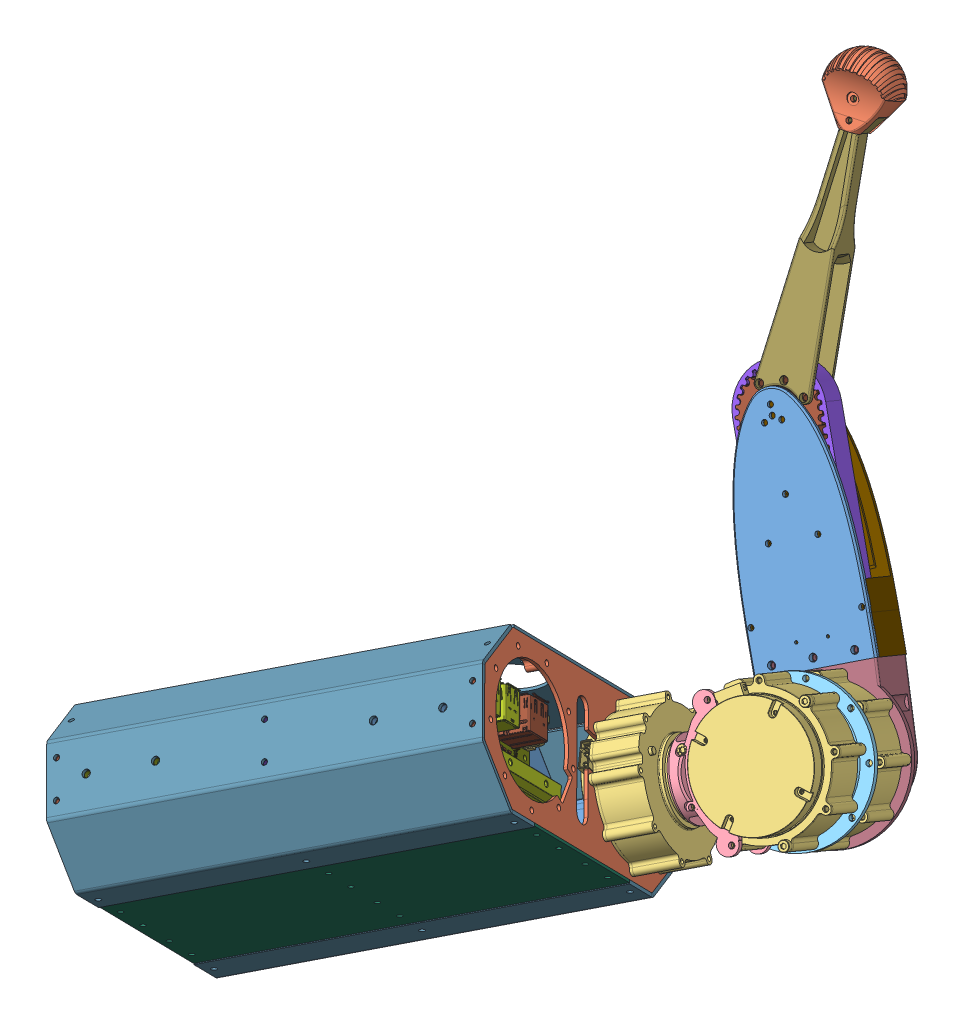
SolidWorks assembly OpenPaws, configuration 默认. Lengths in mm.
Overall size (320.72 417.64 440.55).
429 component instances, 92 part files, 82 mates.
Components (placement in the parent):
- BackFrame-1: BackFrame [默认] at (73.8698 29.661 407.5892) x (-0.005778 -0.713341 -0.700793) z (0.575051 -0.575706 0.581273) size (175.11 55 85)
- Shoulder-1: Shoulder [默认] at (126.526 -8.5635 317.638) x (0.005778 0.713341 0.700793) z (0.575051 -0.575706 0.581273) size (175 10 85)
- Shoulder-2: Shoulder [默认] at (-52.9353 -32.2821 471.687) x (-0.005778 -0.713341 -0.700793) z (0.575051 -0.575706 0.581273) size (175 10 85)
- GearMotor-2: GearMotor [默认] at (151.3659 -129.7436 299.245) x (0.045262 0.672114 0.739063) z (-0.818097 -0.399633 0.413534) size (79.28 79.04 36.5)
- BodyLink-1: BodyLink [默认] at (206.2936 -47.6345 302.2147) x (0.743726 -0.643745 0.180177) z (-0.637204 -0.601205 0.482206) size (72.12 36.71 41.06)
- GearMotor-3: GearMotor [默认] at (304.5713 -13.1331 316.7999) x (-0.480926 0.810551 -0.33424) z (0.202095 0.473439 0.857329) size (79.28 79.04 36.5)
- HipLink-1: HipLink [默认] at (180.5751 12.35 275.3856) x (-0.719619 0.665567 -0.19791) z (-0.664309 -0.576954 0.475203) size (80.5 13.5 80.5)
- GearMotor-6: GearMotor [默认] at (287.2301 -48.9231 292.2457) x (-0.325496 0.8581 -0.397136) z (0.202095 0.473439 0.857329) size (79.28 79.04 36.5)
- HipGearGuard-3: HipGearGuard [默认] at (172.1585 -9.0925 236.1389) x (-0.439258 -0.738587 0.511411) z (0.202095 0.473439 0.857329) size (50 50 4)
- HipGear-1: HipGear [默认] at (169.127 -16.194 223.2789) x (-0.439258 -0.738587 0.511411) z (0.202095 0.473439 0.857329) size (43.22 43.22 15)
- HipGearGuard-4: HipGearGuard [默认] at (169.127 -16.194 223.2789) x (0.977691 -0.046349 -0.204872) z (-0.202095 -0.473439 -0.857329) size (50 50 4)
- Belt-1: Belt [默认] at (170.6529 -12.6221 229.6948) x (-0.202095 -0.473439 -0.857329) z (0.539183 -0.784569 0.306159) size (15 46.9 201.91)
- KneeLink-1: KneeLink [默认] at (90.331 112.9224 193.1849) x (0.876516 -0.477948 0.057317) z (-0.202095 -0.473439 -0.857329) size (20.8 20.8 29)
- KneeBearing-1: KneeBearing [默认] at (89.5016 110.9794 189.6665) x (0.724532 0.516716 -0.456134) z (0.202095 0.473439 0.857329) size (23 23 4)
- KneeBearing-2: KneeBearing [默认] at (85.4395 101.4633 172.4342) x (0.724532 0.516716 -0.456134) z (0.202095 0.473439 0.857329) size (23 23 4)
- KneeGear-1: KneeGear [默认] at (107.8423 104.8503 171.5697) x (0.970121 0.023224 -0.241508) z (0.202095 0.473439 0.857329) size (43.22 43.22 23)
- LowerLink-1: LowerLink [默认] at (80.2616 167.6072 157.9955) x (-0.13425 0.880521 -0.454599) z (-0.970121 -0.023224 0.241508) size (141.69 21.45 28.63)
- HipCover-2: HipCover [默认] at (236.5323 -46.6268 249.8566) x (0.328008 -0.857556 0.396244) z (-0.202095 -0.473439 -0.857329) size (95.72 81 30.11)
- Side Panel-1: Side Panel [默认] at (126.93 41.3087 366.6329) x (0.005778 0.713341 0.700793) z (0.575051 -0.575706 0.581273) size (46.9 220 87.71)
- TopSidePanel-1: TopSidePanel [默认] at (25.87 -62.2266 439.7634) x (0.818097 0.399633 -0.413534) z (0.005778 0.713341 0.700793) size (220 1.5 85.2)
- Side Panel-2: Side Panel [默认] at (-53.3368 -82.1597 422.6916) x (-0.005778 -0.713341 -0.700793) z (0.575051 -0.575706 0.581273) size (46.9 220 87.71)
- Jetson nano.step-1: Jetson nano.step [默认] at (68.0286 -15.5875 328.1241) x (0.005778 0.713341 0.700793) z (0.818097 0.399633 -0.413534) size (100 81.03 30.51)
  - 142-13449-1000-A02_ASM.step-1: 142-13449-1000-A02_ASM.step [默认] at origin size (100 81.03 23.18)
    - 142-13449-1000-A02.step-1: 142-13449-1000-A02.step [默认] at origin size (100 79 1.57)
    - 315-1109-000_1.step-1: 315-1109-000_1.step [默认] at (5.6 4.9 1.575) x (-1 0 0) z (0 0 1) size (4.5 3.5 0.8)
    - 0402_H040.step-1: 0402_H040.step [默认] at (8 -0.825 1.575) size (1 0.5 0.4)
    - 0402_H060.step-1: 0402_H060.step [默认] at (1 5 1.575) x (0 -1 0) z (0 0 1) size (1 0.5 0.6)
    - 0402_H040.step-2: 0402_H040.step [默认] at (9.9 -0.3 1.575) size (1 0.5 0.4)
    - 0402_H040.step-3: 0402_H040.step [默认] at (8.296 51.194 1.575) x (-1 0 0) z (0 0 1) size (1 0.5 0.4)
    - 0402_H040.step-4: 0402_H040.step [默认] at (76.2 36.9 1.575) x (-1 0 0) z (0 0 1) size (1 0.5 0.4)
    - 0402_H040.step-5: 0402_H040.step [默认] at (37.8 2.87 1.575) x (0 -1 0) z (0 0 1) size (1 0.5 0.4)
    - 0402_H040.step-6: 0402_H040.step [默认] at (38.6 2.87 1.575) x (0 -1 0) z (0 0 1) size (1 0.5 0.4)
    - 0402_H060.step-2: 0402_H060.step [默认] at (14.2 7.7 1.575) x (0 -1 0) z (0 0 1) size (1 0.5 0.6)
    - 0402_H040.step-7: 0402_H040.step [默认] at (64 27.5 1.575) x (-1 0 0) z (0 0 1) size (1 0.5 0.4)
    - 0402_H060.step-3: 0402_H060.step [默认] at (18.6 43.15 1.575) x (-1 0 0) z (0 0 1) size (1 0.5 0.6)
    - 0402_H060.step-4: 0402_H060.step [默认] at (65.5 52.8 1.575) x (0 1 0) z (0 0 1) size (1 0.5 0.6)
    - 0402_H060.step-5: 0402_H060.step [默认] at (64 28.4 1.575) x (-1 0 0) z (0 0 1) size (1 0.5 0.6)
    - 0402_H040.step-8: 0402_H040.step [默认] at (60.95 25.85 1.575) size (1 0.5 0.4)
    - 0402_H060.step-6: 0402_H060.step [默认] at (17.3 7.7 1.575) x (0 -1 0) z (0 0 1) size (1 0.5 0.6)
    - 0402_H060.step-7: 0402_H060.step [默认] at (18.6 7.7 1.575) x (0 -1 0) z (0 0 1) size (1 0.5 0.6)
    - 0402_H060.step-8: 0402_H060.step [默认] at (12.9 7.7 1.575) x (0 -1 0) z (0 0 1) size (1 0.5 0.6)
    - 0402_H060.step-9: 0402_H060.step [默认] at (80.9 37.7 1.575) x (-1 0 0) z (0 0 1) size (1 0.5 0.6)
    - 0402_H040.step-9: 0402_H040.step [默认] at (79.5 31.3 1.575) size (1 0.5 0.4)
    - 0402_H040.step-10: 0402_H040.step [默认] at (81 31.3 1.575) x (-1 0 0) z (0 0 1) size (1 0.5 0.4)
    - 0402_H060.step-10: 0402_H060.step [默认] at (79.3 37.7 1.575) size (1 0.5 0.6)
    - 0402_H060.step-11: 0402_H060.step [默认] at (74.8 4.05 1.575) x (-1 0 0) z (0 0 1) size (1 0.5 0.6)
    - 0402_H040.step-11: 0402_H040.step [默认] at (65.675 6.15 1.575) x (0 -1 0) z (0 0 1) size (1 0.5 0.4)
    - 0402_H060.step-12: 0402_H060.step [默认] at (67.7 6.85 1.575) x (0 1 0) z (0 0 1) size (1 0.5 0.6)
    - 0402_H040.step-12: 0402_H040.step [默认] at (64.475 5.8 1.575) x (-1 0 0) z (0 0 1) size (1 0.5 0.4)
    - 0402_H040.step-13: 0402_H040.step [默认] at (67.725 5.325 1.575) x (0 1 0) z (0 0 1) size (1 0.5 0.4)
    - 0402_H060.step-13: 0402_H060.step [默认] at (46.1 59.45 1.575) size (1 0.5 0.6)
    - 0402_H040.step-14: 0402_H040.step [默认] at (44.65 59.45 1.575) size (1 0.5 0.4)
    - 0402_H040.step-15: 0402_H040.step [默认] at (46.1 60.25 1.575) size (1 0.5 0.4)
    - 0402_H060.step-14: 0402_H060.step [默认] at (53.35 57.7 1.575) x (0 -1 0) z (0 0 1) size (1 0.5 0.6)
    - 0402_H040.step-16: 0402_H040.step [默认] at (47.6 59.45 1.575) size (1 0.5 0.4)
    - 0402_H040.step-17: 0402_H040.step [默认] at (48.4 60.25 1.575) size (1 0.5 0.4)
    - 0402_H040.step-18: 0402_H040.step [默认] at (47.7 58.325 1.575) x (0 1 0) z (0 0 1) size (1 0.5 0.4)
    - 0402_H060.step-15: 0402_H060.step [默认] at (46.5 58.65 1.575) x (-1 0 0) z (0 0 1) size (1 0.5 0.6)
    - 0402_H060.step-16: 0402_H060.step [默认] at (51.8 60.25 1.575) size (1 0.5 0.6)
    - 0402_H040.step-19: 0402_H040.step [默认] at (53.35 59.4 1.575) x (0 -1 0) z (0 0 1) size (1 0.5 0.4)
    - 0402_H040.step-20: 0402_H040.step [默认] at (50.2 60.25 1.575) x (-1 0 0) z (0 0 1) size (1 0.5 0.4)
    - 0402_H060.step-17: 0402_H060.step [默认] at (18.6 43.95 1.575) x (-1 0 0) z (0 0 1) size (1 0.5 0.6)
    - 0402_H060.step-18: 0402_H060.step [默认] at (52.75 2.9 1.575) x (0 -1 0) z (0 0 1) size (1 0.5 0.6)
    - 0402_H060.step-19: 0402_H060.step [默认] at (22.35 47.4 1.575) x (-1 0 0) z (0 0 1) size (1 0.5 0.6)
    - 0402_H060.step-20: 0402_H060.step [默认] at (20.55 47.4 1.575) x (-1 0 0) z (0 0 1) size (1 0.5 0.6)
    - 0402_H060.step-21: 0402_H060.step [默认] at (21.95 34.55 1.575) x (0 -1 0) z (0 0 1) size (1 0.5 0.6)
    - 0402_H060.step-22: 0402_H060.step [默认] at (21.05 34.55 1.575) x (0 -1 0) z (0 0 1) size (1 0.5 0.6)
    - 0402_H060.step-23: 0402_H060.step [默认] at (53.55 2.9 1.575) x (0 -1 0) z (0 0 1) size (1 0.5 0.6)
    - 0402_H060.step-24: 0402_H060.step [默认] at (25.4 54 1.575) x (-1 0 0) z (0 0 1) size (1 0.5 0.6)
    - 0402_H060.step-25: 0402_H060.step [默认] at (24 34.58 1.575) x (0 -1 0) z (0 0 1) size (1 0.5 0.6)
    - 0402_H040.step-21: 0402_H040.step [默认] at (55.6 2.95 1.575) x (0 -1 0) z (0 0 1) size (1 0.5 0.4)
    - 0402_H040.step-22: 0402_H040.step [默认] at (20.13 34.53 1.575) x (0 1 0) z (0 0 1) size (1 0.5 0.4)
    - 0402_H060.step-26: 0402_H060.step [默认] at (18.4 35.15 1.575) x (0 1 0) z (0 0 1) size (1 0.5 0.6)
    - 0402_H060.step-27: 0402_H060.step [默认] at (18.4 36.75 1.575) x (0 1 0) z (0 0 1) size (1 0.5 0.6)
    - 0402_H040.step-23: 0402_H040.step [默认] at (39.6 2.87 1.575) x (0 -1 0) z (0 0 1) size (1 0.5 0.4)
    - 0402_H040.step-24: 0402_H040.step [默认] at (40.4 2.87 1.575) x (0 -1 0) z (0 0 1) size (1 0.5 0.4)
    - 0402_H040.step-25: 0402_H040.step [默认] at (60.95 2.95 1.575) x (0 -1 0) z (0 0 1) size (1 0.5 0.4)
    - 0402_H040.step-26: 0402_H040.step [默认] at (60.15 2.95 1.575) x (0 -1 0) z (0 0 1) size (1 0.5 0.4)
    - 0402_H040.step-27: 0402_H040.step [默认] at (54.8 2.95 1.575) x (0 -1 0) z (0 0 1) size (1 0.5 0.4)
    - 0402_H040.step-28: 0402_H040.step [默认] at (31.6 54 1.575) size (1 0.5 0.4)
    - 0402_H040.step-29: 0402_H040.step [默认] at (27.4 54 1.575) size (1 0.5 0.4)
    - 0402_H040.step-30: 0402_H040.step [默认] at (29.6 54 1.575) x (-1 0 0) z (0 0 1) size (1 0.5 0.4)
    - 0402_H040.step-31: 0402_H040.step [默认] at (63.775 -14.475 1.575) size (1 0.5 0.4)
    - 0402_H040.step-32: 0402_H040.step [默认] at (63.775 -15.275 1.575) size (1 0.5 0.4)
    - 0402_H040.step-33: 0402_H040.step [默认] at (8.025 41.475 1.575) x (-1 0 0) z (0 0 1) size (1 0.5 0.4)
    - 0402_H060.step-28: 0402_H060.step [默认] at (63.95 1.25 1.575) x (0 1 0) z (0 0 1) size (1 0.5 0.6)
    - 0402_H060.step-29: 0402_H060.step [默认] at (2.95 54.05 1.575) x (0 1 0) z (0 0 1) size (1 0.5 0.6)
    - 0402_H040.step-34: 0402_H040.step [默认] at (92.2 -3.45 1.575) x (-1 0 0) z (0 0 1) size (1 0.5 0.4)
    - 0402_H060.step-30: 0402_H060.step [默认] at (32.85 7.7 1.575) x (0 -1 0) z (0 0 1) size (1 0.5 0.6)
    - 0402_H060.step-31: 0402_H060.step [默认] at (27.25 7.7 1.575) x (0 -1 0) z (0 0 1) size (1 0.5 0.6)
    - 0402_H060.step-32: 0402_H060.step [默认] at (31.25 7.7 1.575) x (0 -1 0) z (0 0 1) size (1 0.5 0.6)
    - 0402_H060.step-33: 0402_H060.step [默认] at (28.85 7.7 1.575) x (0 -1 0) z (0 0 1) size (1 0.5 0.6)
    - 0402_H060.step-34: 0402_H060.step [默认] at (32.05 7.7 1.575) x (0 -1 0) z (0 0 1) size (1 0.5 0.6)
    - 0402_H060.step-35: 0402_H060.step [默认] at (28.05 7.7 1.575) x (0 -1 0) z (0 0 1) size (1 0.5 0.6)
    - 0402_H060.step-36: 0402_H060.step [默认] at (30.45 7.7 1.575) x (0 -1 0) z (0 0 1) size (1 0.5 0.6)
    - 0402_H060.step-37: 0402_H060.step [默认] at (29.65 7.7 1.575) x (0 -1 0) z (0 0 1) size (1 0.5 0.6)
    - 0402_H060.step-38: 0402_H060.step [默认] at (24.65 6.41 1.575) x (0 -1 0) z (0 0 1) size (1 0.5 0.6)
    - 0402_H060.step-39: 0402_H060.step [默认] at (25.85 6.41 1.575) x (0 -1 0) z (0 0 1) size (1 0.5 0.6)
    - 0402_H060.step-40: 0402_H060.step [默认] at (4.2 36.5 1.575) x (0 1 0) z (0 0 1) size (1 0.5 0.6)
    - 0402_H060.step-41: 0402_H060.step [默认] at (89.7 4.7 1.575) x (0 -1 0) z (0 0 1) size (1 0.5 0.6)
    - 0402_H060.step-42: 0402_H060.step [默认] at (82.5 3.8 1.575) x (0 -1 0) z (0 0 1) size (1 0.5 0.6)
    - 0402_H060.step-43: 0402_H060.step [默认] at (12.65 49.7 1.575) size (1 0.5 0.6)
    - 0402_H060.step-44: 0402_H060.step [默认] at (11.2 50.15 1.575) x (0 -1 0) z (0 0 1) size (1 0.5 0.6)
    - 0402_H060.step-45: 0402_H060.step [默认] at (26.5 34.55 1.575) x (0 -1 0) z (0 0 1) size (1 0.5 0.6)
    - 0402_H060.step-46: 0402_H060.step [默认] at (29.9 34.5 1.575) x (0 -1 0) z (0 0 1) size (1 0.5 0.6)
    - 0402_H060.step-47: 0402_H060.step [默认] at (31.7 40.15 1.575) x (0 1 0) z (0 0 1) size (1 0.5 0.6)
    - 0402_H060.step-48: 0402_H060.step [默认] at (31.15 42.5 1.575) x (0 1 0) z (0 0 1) size (1 0.5 0.6)
    - 0402_H060.step-49: 0402_H060.step [默认] at (19.2 47.05 1.575) x (0 1 0) z (0 0 1) size (1 0.5 0.6)
    - 0402_H060.step-50: 0402_H060.step [默认] at (17.95 42 1.575) x (0 -1 0) z (0 0 1) size (1 0.5 0.6)
    - 0402_H060.step-51: 0402_H060.step [默认] at (27.3 48.25 1.575) x (0 1 0) z (0 0 1) size (1 0.5 0.6)
    - 0402_H060.step-52: 0402_H060.step [默认] at (31.7 37.85 1.575) x (0 -1 0) z (0 0 1) size (1 0.5 0.6)
    - 0402_H060.step-53: 0402_H060.step [默认] at (29.6 48.35 1.575) x (0 1 0) z (0 0 1) size (1 0.5 0.6)
    - 0402_H060.step-54: 0402_H060.step [默认] at (18.8 38.75 1.575) x (-1 0 0) z (0 0 1) size (1 0.5 0.6)
    - 0402_H060.step-55: 0402_H060.step [默认] at (18.7 57.2 1.575) x (0 -1 0) z (0 0 1) size (1 0.5 0.6)
    - 0402_H060.step-56: 0402_H060.step [默认] at (34.1 2.9 1.575) x (0 -1 0) z (0 0 1) size (1 0.5 0.6)
    - 0402_H060.step-57: 0402_H060.step [默认] at (35.8 2.9 1.575) x (0 -1 0) z (0 0 1) size (1 0.5 0.6)
    - 0402_H060.step-58: 0402_H060.step [默认] at (34.9 2.9 1.575) x (0 -1 0) z (0 0 1) size (1 0.5 0.6)
    - 0402_H060.step-59: 0402_H060.step [默认] at (36.6 2.9 1.575) x (0 -1 0) z (0 0 1) size (1 0.5 0.6)
    - 0402_H060.step-60: 0402_H060.step [默认] at (11.325 44.725 1.575) size (1 0.5 0.6)
    - 0402_H060.step-61: 0402_H060.step [默认] at (50.95 2.9 1.575) x (0 -1 0) z (0 0 1) size (1 0.5 0.6)
    - 0402_H060.step-62: 0402_H060.step [默认] at (51.75 2.9 1.575) x (0 -1 0) z (0 0 1) size (1 0.5 0.6)
    - 0402_H060.step-63: 0402_H060.step [默认] at (11.55 39.7 1.575) size (1 0.5 0.6)
    - 0402_H060.step-64: 0402_H060.step [默认] at (9.5 -8.5 1.575) x (-1 0 0) z (0 0 1) size (1 0.5 0.6)
    - 0402_H060.step-65: 0402_H060.step [默认] at (61.35 38.05 1.575) x (0 -1 0) z (0 0 1) size (1 0.5 0.6)
    - 0402_H060.step-66: 0402_H060.step [默认] at (60.55 38.05 1.575) x (0 -1 0) z (0 0 1) size (1 0.5 0.6)
    - 0402_H060.step-67: 0402_H060.step [默认] at (29.3 25.65 1.575) x (0 -1 0) z (0 0 1) size (1 0.5 0.6)
    - 0402_H060.step-68: 0402_H060.step [默认] at (63.3 56.2 1.575) x (0 1 0) z (0 0 1) size (1 0.5 0.6)
    - 0402_H060.step-69: 0402_H060.step [默认] at (20.5 54.2 1.575) size (1 0.5 0.6)
    - 0402_H060.step-70: 0402_H060.step [默认] at (60.1 32.15 1.575) x (0 1 0) z (0 0 1) size (1 0.5 0.6)
    - 0402_H060.step-71: 0402_H060.step [默认] at (60.9 32.15 1.575) x (0 1 0) z (0 0 1) size (1 0.5 0.6)
    - 0402_H060.step-72: 0402_H060.step [默认] at (18.6 44.85 1.575) size (1 0.5 0.6)
    - 0402_H060.step-73: 0402_H060.step [默认] at (18.6 45.65 1.575) size (1 0.5 0.6)
    - 0402_H060.step-74: 0402_H060.step [默认] at (18.1 27.25 1.575) size (1 0.5 0.6)
    - 0402_H060.step-75: 0402_H060.step [默认] at (15.1 7.7 1.575) x (0 -1 0) z (0 0 1) size (1 0.5 0.6)
    - 0402_H060.step-76: 0402_H060.step [默认] at (16.4 7.7 1.575) x (0 -1 0) z (0 0 1) size (1 0.5 0.6)
    - 0402_H060.step-77: 0402_H060.step [默认] at (20.8 7.7 1.575) x (0 -1 0) z (0 0 1) size (1 0.5 0.6)
    - 0402_H060.step-78: 0402_H060.step [默认] at (19.5 7.7 1.575) x (0 -1 0) z (0 0 1) size (1 0.5 0.6)
    - 0402_H060.step-79: 0402_H060.step [默认] at (21.9 2.8 1.575) size (1 0.5 0.6)
    - 0402_H060.step-80: 0402_H060.step [默认] at (12.75 29 1.575) size (1 0.5 0.6)
    - 0402_H060.step-81: 0402_H060.step [默认] at (10.225 5.1 1.575) size (1 0.5 0.6)
    - 0402_H060.step-82: 0402_H060.step [默认] at (22.8 27.65 1.575) x (0 1 0) z (0 0 1) size (1 0.5 0.6)
    - 0402_H060.step-83: 0402_H060.step [默认] at (18.85 25.15 1.575) x (0 -1 0) z (0 0 1) size (1 0.5 0.6)
    - 0402_H060.step-84: 0402_H060.step [默认] at (17.95 40.1 1.575) x (0 1 0) z (0 0 1) size (1 0.5 0.6)
    - 0402_H040.step-35: 0402_H040.step [默认] at (20.8 6.2 1.575) x (0 1 0) z (0 0 1) size (1 0.5 0.4)
    - 0402_H040.step-36: 0402_H040.step [默认] at (76 22.7 1.575) size (1 0.5 0.4)
    - 0402_H040.step-37: 0402_H040.step [默认] at (23.7 26.85 1.575) x (0 1 0) z (0 0 1) size (1 0.5 0.4)
    - 0402_H040.step-38: 0402_H040.step [默认] at (18 25.15 1.575) x (0 1 0) z (0 0 1) size (1 0.5 0.4)
    - 0402_H040.step-39: 0402_H040.step [默认] at (17.3 28.25 1.575) x (-1 0 0) z (0 0 1) size (1 0.5 0.4)
    - 0402_H040.step-40: 0402_H040.step [默认] at (13.15 4.2 1.575) x (0 -1 0) z (0 0 1) size (1 0.5 0.4)
    - 0402_H040.step-41: 0402_H040.step [默认] at (17.2 30.15 1.575) x (0 -1 0) z (0 0 1) size (1 0.5 0.4)
    - 0402_H040.step-42: 0402_H040.step [默认] at (14.2 6.2 1.575) x (0 1 0) z (0 0 1) size (1 0.5 0.4)
    - 0402_H040.step-43: 0402_H040.step [默认] at (12.9 6.2 1.575) x (0 1 0) z (0 0 1) size (1 0.5 0.4)
    - 0402_H040.step-44: 0402_H040.step [默认] at (15.1 6.2 1.575) x (0 1 0) z (0 0 1) size (1 0.5 0.4)
    - 0402_H040.step-45: 0402_H040.step [默认] at (16.4 6.2 1.575) x (0 1 0) z (0 0 1) size (1 0.5 0.4)
    - 0402_H040.step-46: 0402_H040.step [默认] at (19.5 6.2 1.575) x (0 1 0) z (0 0 1) size (1 0.5 0.4)
    - 0402_H040.step-47: 0402_H040.step [默认] at (17.3 6.2 1.575) x (0 1 0) z (0 0 1) size (1 0.5 0.4)
    - 0402_H040.step-48: 0402_H040.step [默认] at (18.6 6.2 1.575) x (0 1 0) z (0 0 1) size (1 0.5 0.4)
    - 0402_H040.step-49: 0402_H040.step [默认] at (24.2 24.55 1.575) x (0 1 0) z (0 0 1) size (1 0.5 0.4)
    - 0402_H040.step-50: 0402_H040.step [默认] at (23.5 54.9 1.575) x (0 1 0) z (0 0 1) size (1 0.5 0.4)
    - 0402_H040.step-51: 0402_H040.step [默认] at (13.2 39.75 1.575) x (-1 0 0) z (0 0 1) size (1 0.5 0.4)
    - 0402_H040.step-52: 0402_H040.step [默认] at (80.7 47.4 1.575) x (-1 0 0) z (0 0 1) size (1 0.5 0.4)
    - 0402_H040.step-53: 0402_H040.step [默认] at (77.5 22.7 1.575) x (-1 0 0) z (0 0 1) size (1 0.5 0.4)
    - 0402_H040.step-54: 0402_H040.step [默认] at (9.25 -12.75 1.575) x (-1 0 0) z (0 0 1) size (1 0.5 0.4)
    - 0402_H040.step-55: 0402_H040.step [默认] at (9.25 -11.95 1.575) x (-1 0 0) z (0 0 1) size (1 0.5 0.4)
    - 0402_H040.step-56: 0402_H040.step [默认] at (64.475 6.7 1.575) size (1 0.5 0.4)
    - 0402_H040.step-57: 0402_H040.step [默认] at (29.3 24 1.575) x (0 1 0) z (0 0 1) size (1 0.5 0.4)
    - 0402_H040.step-58: 0402_H040.step [默认] at (64.2 32.5 1.575) x (0 1 0) z (0 0 1) size (1 0.5 0.4)
    - 0402_H040.step-59: 0402_H040.step [默认] at (64.15 47.45 1.575) x (0 -1 0) z (0 0 1) size (1 0.5 0.4)
    - 0402_H040.step-60: 0402_H040.step [默认] at (64.2 31 1.575) x (0 -1 0) z (0 0 1) size (1 0.5 0.4)
    - 0402_H040.step-61: 0402_H040.step [默认] at (76.2 36.1 1.575) x (-1 0 0) z (0 0 1) size (1 0.5 0.4)
    - 0402_H040.step-62: 0402_H040.step [默认] at (78.4 45.15 1.575) size (1 0.5 0.4)
    - 0402_H040.step-63: 0402_H040.step [默认] at (81.7 38.6 1.575) size (1 0.5 0.4)
    - 0402_H040.step-64: 0402_H040.step [默认] at (81.7 39.4 1.575) size (1 0.5 0.4)
    - 0402_H040.step-65: 0402_H040.step [默认] at (59.35 51.825 1.575) size (1 0.5 0.4)
    - 0402_H040.step-66: 0402_H040.step [默认] at (60.825 51.825 1.575) x (-1 0 0) z (0 0 1) size (1 0.5 0.4)
    - 0402_H040.step-67: 0402_H040.step [默认] at (89.7 9.5 1.575) x (0 1 0) z (0 0 1) size (1 0.5 0.4)
    - 0402_H040.step-68: 0402_H040.step [默认] at (89.7 6.7 1.575) x (0 1 0) z (0 0 1) size (1 0.5 0.4)
    - 0402_H040.step-69: 0402_H040.step [默认] at (3.9 34.2 1.575) x (0 -1 0) z (0 0 1) size (1 0.5 0.4)
    - 0402_H040.step-70: 0402_H040.step [默认] at (5.1 35 1.575) x (0 1 0) z (0 0 1) size (1 0.5 0.4)
    - 0402_H040.step-71: 0402_H040.step [默认] at (32.85 5.81 1.575) x (0 -1 0) z (0 0 1) size (1 0.5 0.4)
    - 0402_H040.step-72: 0402_H040.step [默认] at (32.05 5.81 1.575) x (0 -1 0) z (0 0 1) size (1 0.5 0.4)
    - 0402_H040.step-73: 0402_H040.step [默认] at (27.25 5.81 1.575) x (0 -1 0) z (0 0 1) size (1 0.5 0.4)
    - 0402_H040.step-74: 0402_H040.step [默认] at (28.05 5.81 1.575) x (0 -1 0) z (0 0 1) size (1 0.5 0.4)
    - 0402_H040.step-75: 0402_H040.step [默认] at (31.25 5.81 1.575) x (0 -1 0) z (0 0 1) size (1 0.5 0.4)
    - 0402_H040.step-76: 0402_H040.step [默认] at (30.45 5.81 1.575) x (0 -1 0) z (0 0 1) size (1 0.5 0.4)
    - 0402_H040.step-77: 0402_H040.step [默认] at (28.85 5.81 1.575) x (0 -1 0) z (0 0 1) size (1 0.5 0.4)
    - 0402_H040.step-78: 0402_H040.step [默认] at (29.65 5.81 1.575) x (0 -1 0) z (0 0 1) size (1 0.5 0.4)
    - 0402_H040.step-79: 0402_H040.step [默认] at (13.5 52.9 1.575) x (-1 0 0) z (0 0 1) size (1 0.5 0.4)
    - 0402_H040.step-80: 0402_H040.step [默认] at (22.35 4 1.575) x (0 -1 0) z (0 0 1) size (1 0.5 0.4)
    - 0402_H040.step-81: 0402_H040.step [默认] at (21.55 4 1.575) x (0 1 0) z (0 0 1) size (1 0.5 0.4)
    - 0402_H040.step-82: 0402_H040.step [默认] at (25.85 4.9 1.575) x (0 -1 0) z (0 0 1) size (1 0.5 0.4)
    - 0402_H040.step-83: 0402_H040.step [默认] at (11.8 52.9 1.575) size (1 0.5 0.4)
    - 0402_H040.step-84: 0402_H040.step [默认] at (9.432 51.594 1.575) x (0 -1 0) z (0 0 1) size (1 0.5 0.4)
    - 0402_H040.step-85: 0402_H040.step [默认] at (8.975 50.3 1.575) size (1 0.5 0.4)
    - 0402_H040.step-86: 0402_H040.step [默认] at (82.8 -5.3 1.575) x (-1 0 0) z (0 0 1) size (1 0.5 0.4)
    - 0402_H040.step-87: 0402_H040.step [默认] at (82.4 -11.6 1.575) x (-1 0 0) z (0 0 1) size (1 0.5 0.4)
    - 0402_H040.step-88: 0402_H040.step [默认] at (22.8 26.05 1.575) x (0 1 0) z (0 0 1) size (1 0.5 0.4)
    - 0402_H040.step-89: 0402_H040.step [默认] at (20.8 28.25 1.575) size (1 0.5 0.4)
    - 0402_H040.step-90: 0402_H040.step [默认] at (20.8 24.65 1.575) x (-1 0 0) z (0 0 1) size (1 0.5 0.4)
    - 0402_H040.step-91: 0402_H040.step [默认] at (18.1 26.45 1.575) size (1 0.5 0.4)
    - 0402_H040.step-92: 0402_H040.step [默认] at (24.65 8.41 1.575) x (0 1 0) z (0 0 1) size (1 0.5 0.4)
    - 0402_H040.step-93: 0402_H040.step [默认] at (25.85 8.41 1.575) x (0 1 0) z (0 0 1) size (1 0.5 0.4)
    - 0402_H040.step-94: 0402_H040.step [默认] at (3.8 54.4 1.575) x (0 -1 0) z (0 0 1) size (1 0.5 0.4)
    - 0402_H040.step-95: 0402_H040.step [默认] at (2.45 44.45 1.575) x (0 -1 0) z (0 0 1) size (1 0.5 0.4)
    - 0402_H040.step-96: 0402_H040.step [默认] at (24.65 4.9 1.575) x (0 1 0) z (0 0 1) size (1 0.5 0.4)
    - 0402_H040.step-97: 0402_H040.step [默认] at (22.15 7.6 1.575) x (-1 0 0) z (0 0 1) size (1 0.5 0.4)
    - 0402_H040.step-98: 0402_H040.step [默认] at (79.2 47.4 1.575) size (1 0.5 0.4)
    - 0402_H040.step-99: 0402_H040.step [默认] at (19 28.25 1.575) size (1 0.5 0.4)
    - 0402_H040.step-100: 0402_H040.step [默认] at (9.65 9.7 1.575) x (0 -1 0) z (0 0 1) size (1 0.5 0.4)
    - 0402_H040.step-101: 0402_H040.step [默认] at (28.35 34.45 1.575) x (0 1 0) z (0 0 1) size (1 0.5 0.4)
    - 0402_H040.step-102: 0402_H040.step [默认] at (25.2 34.55 1.575) x (0 1 0) z (0 0 1) size (1 0.5 0.4)
    - 0402_H040.step-103: 0402_H040.step [默认] at (10.625 6.35 1.575) x (0 -1 0) z (0 0 1) size (1 0.5 0.4)
    - 0402_H040.step-104: 0402_H040.step [默认] at (9.825 6.35 1.575) x (0 1 0) z (0 0 1) size (1 0.5 0.4)
    - 0402_H040.step-105: 0402_H040.step [默认] at (4.775 42.975 1.575) x (0 1 0) z (0 0 1) size (1 0.5 0.4)
    - 0402_H040.step-106: 0402_H040.step [默认] at (19.8 32.9 1.575) x (-1 0 0) z (0 0 1) size (1 0.5 0.4)
    - 0402_H040.step-107: 0402_H040.step [默认] at (22.35 24.65 1.575) x (-1 0 0) z (0 0 1) size (1 0.5 0.4)
    - 0402_H040.step-108: 0402_H040.step [默认] at (62.4 54.7 1.575) size (1 0.5 0.4)
    - 0402_H040.step-109: 0402_H040.step [默认] at (62.2 60.05 1.575) x (-1 0 0) z (0 0 1) size (1 0.5 0.4)
    - 0402_H040.step-110: 0402_H040.step [默认] at (23.5 57.5 1.575) x (0 1 0) z (0 0 1) size (1 0.5 0.4)
    - 0402_H040.step-111: 0402_H040.step [默认] at (12.8 44.725 1.575) size (1 0.5 0.4)
    - 0402_H040.step-112: 0402_H040.step [默认] at (21.8 31.45 1.575) x (0 1 0) z (0 0 1) size (1 0.5 0.4)
    - 0402_H040.step-113: 0402_H040.step [默认] at (19.25 34.55 1.575) x (0 1 0) z (0 0 1) size (1 0.5 0.4)
    - 0402_H040.step-114: 0402_H040.step [默认] at (0.95 41.55 1.575) size (1 0.5 0.4)
    - 0402_H040.step-115: 0402_H040.step [默认] at (64.1 58 1.575) x (0 1 0) z (0 0 1) size (1 0.5 0.4)
    - 0402_H040.step-116: 0402_H040.step [默认] at (63.3 58 1.575) x (0 -1 0) z (0 0 1) size (1 0.5 0.4)
    - 0402_H040.step-117: 0402_H040.step [默认] at (63.55 59.7 1.575) x (0 -1 0) z (0 0 1) size (1 0.5 0.4)
    - 0402_H060.step-85: 0402_H060.step [默认] at (71.175 4 1.575) x (-1 0 0) z (0 0 1) size (1 0.5 0.6)
    - 0402_H040.step-118: 0402_H040.step [默认] at (86.6 -5.6 1.575) x (0 1 0) z (0 0 1) size (1 0.5 0.4)
    - 0402_H040.step-119: 0402_H040.step [默认] at (85.8 -5.3 1.575) x (0 1 0) z (0 0 1) size (1 0.5 0.4)
    - 0402_H040.step-120: 0402_H040.step [默认] at (10.25 51.6 1.575) x (0 1 0) z (0 0 1) size (1 0.5 0.4)
    - 0402_H040.step-121: 0402_H040.step [默认] at (80.5 28.55 1.575) size (1 0.5 0.4)
    - 0402_H040.step-122: 0402_H040.step [默认] at (13.95 4.2 1.575) x (0 -1 0) z (0 0 1) size (1 0.5 0.4)
    - 0402_H040.step-123: 0402_H040.step [默认] at (15.35 4.2 1.575) x (0 -1 0) z (0 0 1) size (1 0.5 0.4)
    - 0402_H040.step-124: 0402_H040.step [默认] at (16.15 4.2 1.575) x (0 -1 0) z (0 0 1) size (1 0.5 0.4)
    - 0402_H040.step-125: 0402_H040.step [默认] at (20.55 4.2 1.575) x (0 -1 0) z (0 0 1) size (1 0.5 0.4)
    - 0402_H040.step-126: 0402_H040.step [默认] at (19.75 4.2 1.575) x (0 -1 0) z (0 0 1) size (1 0.5 0.4)
    - 0402_H040.step-127: 0402_H040.step [默认] at (17.6 4.2 1.575) x (0 -1 0) z (0 0 1) size (1 0.5 0.4)
    - 0402_H040.step-128: 0402_H040.step [默认] at (18.4 4.2 1.575) x (0 -1 0) z (0 0 1) size (1 0.5 0.4)
    - 0402_H060.step-86: 0402_H060.step [默认] at (64.25 -13.325 1.575) x (0 -1 0) z (0 0 1) size (1 0.5 0.6)
    - 0402_H060.step-87: 0402_H060.step [默认] at (64.225 -11.825 1.575) x (0 1 0) z (0 0 1) size (1 0.5 0.6)
    - 0402_H040.step-129: 0402_H040.step [默认] at (63.8 -6.85 1.575) x (0 1 0) z (0 0 1) size (1 0.5 0.4)
    - 0402_H040.step-130: 0402_H040.step [默认] at (81.7 41.95 1.575) size (1 0.5 0.4)
    - 0402_H040.step-131: 0402_H040.step [默认] at (87.75 -6 1.575) x (-1 0 0) z (0 0 1) size (1 0.5 0.4)
    - 0402_H040.step-132: 0402_H040.step [默认] at (82.4 -13.6 1.575) x (-1 0 0) z (0 0 1) size (1 0.5 0.4)
    - 0402_H060.step-88: 0402_H060.step [默认] at (91.75 -5.95 1.575) size (1 0.5 0.6)
    - 0402_H040.step-133: 0402_H040.step [默认] at (3.65 49.25 1.575) x (0 -1 0) z (0 0 1) size (1 0.5 0.4)
    - 0402_H040.step-134: 0402_H040.step [默认] at (2.45 49.25 1.575) x (0 1 0) z (0 0 1) size (1 0.5 0.4)
    - 0402_H040.step-135: 0402_H040.step [默认] at (90.75 -1.45 1.575) x (-1 0 0) z (0 0 1) size (1 0.5 0.4)
    - 0402_H040.step-136: 0402_H040.step [默认] at (8.45 39.55 1.575) x (0 -1 0) z (0 0 1) size (1 0.5 0.4)
    - 0402_H060.step-89: 0402_H060.step [默认] at (8.85 -5.25 1.575) x (-1 0 0) z (0 0 1) size (1 0.5 0.6)
    - 0402_H040.step-137: 0402_H040.step [默认] at (18.6 32.55 1.575) x (0 1 0) z (0 0 1) size (1 0.5 0.4)
    - 0402_H060.step-90: 0402_H060.step [默认] at (4.5 44.45 1.575) x (0 1 0) z (0 0 1) size (1 0.5 0.6)
    - 0402_H040.step-138: 0402_H040.step [默认] at (8.35 2.75 1.575) size (1 0.5 0.4)
    - 0402_H040.step-139: 0402_H040.step [默认] at (9.4 1.95 1.575) size (1 0.5 0.4)
    - 0402_H040.step-140: 0402_H040.step [默认] at (8.2 1.55 1.575) x (0 1 0) z (0 0 1) size (1 0.5 0.4)
    - 0402_H060.step-91: 0402_H060.step [默认] at (8.5 3.875 1.575) x (0 -1 0) z (0 0 1) size (1 0.5 0.6)
    - 0402_H060.step-92: 0402_H060.step [默认] at (-0.8 41.5 1.575) x (-1 0 0) z (0 0 1) size (1 0.5 0.6)
    - 0402_H040.step-141: 0402_H040.step [默认] at (-1.35 7.75 1.575) size (1 0.5 0.4)
    - 0402_H040.step-142: 0402_H040.step [默认] at (8 0.425 1.575) size (1 0.5 0.4)
    - 0402_H040.step-143: 0402_H040.step [默认] at (67.9 4.025 1.575) x (-1 0 0) z (0 0 1) size (1 0.5 0.4)
    - 0402_H040.step-144: 0402_H040.step [默认] at (60.6 60.05 1.575) x (-1 0 0) z (0 0 1) size (1 0.5 0.4)
    - 0402_H040.step-145: 0402_H040.step [默认] at (72.85 4 1.575) x (-1 0 0) z (0 0 1) size (1 0.5 0.4)
    - 0402_H040.step-146: 0402_H040.step [默认] at (64.8 59.35 1.575) size (1 0.5 0.4)
    - 0402_H040.step-147: 0402_H040.step [默认] at (7.2 7.3 1.575) size (1 0.5 0.4)
    - 0402_H040.step-148: 0402_H040.step [默认] at (8.5 5.35 1.575) x (0 1 0) z (0 0 1) size (1 0.5 0.4)
    - 0402_H040.step-149: 0402_H040.step [默认] at (8.475 7.075 1.575) x (0 1 0) z (0 0 1) size (1 0.5 0.4)
    - VIRTUAL_SHORT.step-1: VIRTUAL_SHORT.step [默认] at (23.5 32.9 1.575) x (0 1 0) z (0 0 1) size (0.25 0.25 1)
    - VIRTUAL_SHORT.step-2: VIRTUAL_SHORT.step [默认] at (26.85 32.85 1.575) x (0 1 0) z (0 0 1) size (0.25 0.25 1)
    - VIRTUAL_SHORT.step-3: VIRTUAL_SHORT.step [默认] at (30.6 33.8 1.575) x (0 1 0) z (0 0 1) size (0.25 0.25 1)
    - VIRTUAL_SHORT.step-4: VIRTUAL_SHORT.step [默认] at (32.65 39.75 1.575) x (-1 0 0) z (0 0 1) size (0.25 0.25 1)
    - VIRTUAL_SHORT.step-5: VIRTUAL_SHORT.step [默认] at (31.85 42.1 1.575) x (-1 0 0) z (0 0 1) size (0.25 0.25 1)
    - VIRTUAL_SHORT.step-6: VIRTUAL_SHORT.step [默认] at (17.35 42.4 1.575) size (0.25 0.25 1)
    - VIRTUAL_SHORT.step-7: VIRTUAL_SHORT.step [默认] at (18.6 46.6 1.575) size (0.25 0.25 1)
    - VIRTUAL_SHORT.step-8: VIRTUAL_SHORT.step [默认] at (20.9 32.9 1.575) x (0 1 0) z (0 0 1) size (0.25 0.25 1)
    - VIRTUAL_SHORT.step-9: VIRTUAL_SHORT.step [默认] at (28.6 48.25 1.575) x (0 -1 0) z (0 0 1) size (0.25 0.25 1)
    - VIRTUAL_SHORT.step-10: VIRTUAL_SHORT.step [默认] at (27.1 49.35 1.575) x (0 -1 0) z (0 0 1) size (0.25 0.25 1)
    - VIRTUAL_SHORT.step-11: VIRTUAL_SHORT.step [默认] at (22.1 32.95 1.575) x (-1 0 0) z (0 0 1) size (0.25 0.25 1)
    - VIRTUAL_SHORT.step-12: VIRTUAL_SHORT.step [默认] at (32.65 38.25 1.575) x (-1 0 0) z (0 0 1) size (0.25 0.25 1)
    - VIRTUAL_SHORT.step-13: VIRTUAL_SHORT.step [默认] at (30.3 48 1.575) x (-1 0 0) z (0 0 1) size (0.25 0.25 1)
    - VIRTUAL_SHORT.step-14: VIRTUAL_SHORT.step [默认] at (17.15 38.95 1.575) size (0.25 0.25 1)
    - VIRTUAL_SHORT.step-15: VIRTUAL_SHORT.step [默认] at (17.15 39.7 1.575) size (0.25 0.25 1)
    - VIRTUAL_SHORT.step-16: VIRTUAL_SHORT.step [默认] at (76.175 4.1 1.575) x (-1 0 0) z (0 0 1) size (0.25 0.25 1)
    - 064-0377-000_2.step-1: 064-0377-000_2.step [默认] at (2 -4.75 1.575) x (0 -1 0) z (0 0 1) size (14.63 10.08 14.5)
    - 074-0117-000_2.step-1: 074-0117-000_2.step [默认] at (0.254 14.3 1.575) size (5.08 2.54 11.66)
    - 090-0096-000_1.step-1: 090-0096-000_1.step [默认] at (3.45 44.4 1.575) x (0 -1 0) z (0 0 1) size (1.2 0.6 0.4)
    - 090-0309-000_1.step-1: 090-0309-000_1.step [默认] at (-1.65 8.7 1.575) x (-1 0 0) z (0 0 1) size (1.2 0.6 0.4)
    - 115-1232-000_2.step-1: 115-1232-000_2.step [默认] at (1.25 6.5 1.575) x (-1 0 0) z (0 0 1) size (0.9 0.9 0.33)
    - 074-0102-000_4.step-1: 074-0102-000_4.step [默认] at (0.254 44.36 1.575) x (0 1 0) z (0 0 1) size (10.16 5.08 11.6)
    - 064-0400-000_1.step-1: 064-0400-000_1.step [默认] at (73.75 7.77 1.575) size (10.16 5.8 13.5)
    - MEC_STANDOFF_PTH_620C380P.step-1: MEC_STANDOFF_PTH_620C380P.step [默认] at (40.276 40.3 1.575) x (0 1 0) z (0 0 1) size (6.2 6.2 0.73)
    - 090-0231-000_1.step-1: 090-0231-000_1.step [默认] at (35.3 0.7 1.575) x (-1 0 0) z (0 0 1) size (2.5 1.55 0.55)
    - 090-0231-000_1.step-2: 090-0231-000_1.step [默认] at (52.25 0.7 1.575) x (-1 0 0) z (0 0 1) size (2.5 1.55 0.55)
    - 090-0231-000_1.step-3: 090-0231-000_1.step [默认] at (56.05 0.7 1.575) size (2.5 1.55 0.55)
    - 090-0231-000_1.step-4: 090-0231-000_1.step [默认] at (59.65 0.7 1.575) size (2.5 1.55 0.55)
    - 090-0231-000_1.step-5: 090-0231-000_1.step [默认] at (39.1 0.7 1.575) size (2.5 1.55 0.55)
    - 090-0231-000_1.step-6: 090-0231-000_1.step [默认] at (43.1 0.7 1.575) size (2.5 1.55 0.55)
    - 090-0231-000_1.step-7: 090-0231-000_1.step [默认] at (14.6 1.8 1.575) size (2.5 1.55 0.55)
    - 090-0231-000_1.step-8: 090-0231-000_1.step [默认] at (19.1 1.8 1.575) size (2.5 1.55 0.55)
    - 090-0231-000_1.step-9: 090-0231-000_1.step [默认] at (22.5 1.4 1.575) size (2.5 1.55 0.55)
    - 090-0231-000_1.step-10: 090-0231-000_1.step [默认] at (28.45 3.35 1.575) size (2.5 1.55 0.55)
    - 090-0231-000_1.step-11: 090-0231-000_1.step [默认] at (31.65 3.35 1.575) size (2.5 1.55 0.55)
    - 074-0223-000_2.step-1: 074-0223-000_2.step [默认] at (5.85 53.25 1.575) x (0 1 0) z (0 0 1) size (15.24 2.54 11.6)
    - 131-0832-000_2.step-1: 131-0832-000_2.step [默认] at (56.3 54.7 1.575) x (0 -1 0) z (0 0 1) size (4.96 4.06 1.8)
    - 115-0836-000_1.step-1: 115-0836-000_1.step [默认] at (21.1 56.6 1.575) size (2.9 3.58 1.45)
    - 115-0836-000_1.step-2: 115-0836-000_1.step [默认] at (11.8 42.3 1.575) size (2.9 3.58 1.45)
    - 315-0620-000_1.step-1: 315-0620-000_1.step [默认] at (72.1 53.4 1.575) x (0 -1 0) z (0 0 1) size (2.9 3.58 1.1)
    - 315-1062-000_1.step-1: 315-1062-000_1.step [默认] at (26.8 25.15 1.575) x (0 -1 0) z (0 0 1) size (2.9 3.58 1.45)
    - 170-0285-000_1.step-1: 170-0285-000_1.step [默认] at (28.72 57.28 1.575) x (0 1 0) z (0 0 1) size (4.9 7.21 1.75)
    - 115-0138-000_1.step-1: 115-0138-000_1.step [默认] at (9.15 48.55 1.575) x (0 1 0) z (0 0 1) size (2 2.88 1.1)
    - 115-1821-000_1.step-1: 115-1821-000_1.step [默认] at (3.3 40.8 1.575) x (-1 0 0) z (0 0 1) size (2 2.88 1.1)
    - 115-1821-000_1.step-2: 115-1821-000_1.step [默认] at (6.25 39.55 1.575) x (0 -1 0) z (0 0 1) size (2 2.88 1.1)
    - 115-0742-000_2.step-1: 115-0742-000_2.step [默认] at (3.05 46.85 1.575) size (2 2.88 1.1)
    - 115-0742-000_2.step-2: 115-0742-000_2.step [默认] at (3.05 51.65 1.575) x (-1 0 0) z (0 0 1) size (2 2.88 1.1)
    - 115-1821-000_1.step-3: 115-1821-000_1.step [默认] at (59.6 27.6 1.575) x (0 1 0) z (0 0 1) size (2 2.88 1.1)
    - 091-0022-000_1.step-1: 091-0022-000_1.step [默认] at (-0.95 5.7 1.575) size (2 2.51 1.1)
    - 091-0023-000_1.step-1: 091-0023-000_1.step [默认] at (15.25 29.9 1.575) x (0 -1 0) z (0 0 1) size (2 2.51 1.1)
    - 080-1368-000_1.step-1: 080-1368-000_1.step [默认] at (88 -14.3 1.575) size (10.99 7.28 4.95)
    - 080-1656-000_3.step-1: 080-1656-000_3.step [默认] at (44 16.6 1.575) x (-1 0 0) z (0 0 1) size (77.5 25.85 9.69)
    - 090-0243-000_1.step-1: 090-0243-000_1.step [默认] at (8.5 -4.1 1.575) x (-1 0 0) z (0 0 1) size (1.41 0.61 0.45)
    - 090-0243-000_1.step-2: 090-0243-000_1.step [默认] at (9.95 -3.7 1.575) x (0 1 0) z (0 0 1) size (1.41 0.61 0.45)
    - 090-0243-000_1.step-3: 090-0243-000_1.step [默认] at (9.5 -10.95 1.575) x (-1 0 0) z (0 0 1) size (1.41 0.61 0.45)
    - 090-0243-000_1.step-4: 090-0243-000_1.step [默认] at (9.8 -6.25 1.575) x (-1 0 0) z (0 0 1) size (1.41 0.61 0.45)
    - 090-0243-000_1.step-5: 090-0243-000_1.step [默认] at (9.5 -9.5 1.575) x (-1 0 0) z (0 0 1) size (1.41 0.61 0.45)
    - 090-0172-000_1.step-1: 090-0172-000_1.step [默认] at (90.6 -5 1.575) size (1.41 0.61 0.55)
    - 090-0172-000_1.step-2: 090-0172-000_1.step [默认] at (88.8 -5 1.575) x (-1 0 0) z (0 0 1) size (1.41 0.61 0.55)
    - 115-2177-000_2.step-1: 115-2177-000_2.step [默认] at (12.7 51.35 1.575) x (0 1 0) z (0 0 1) size (1.8 1.71 0.4)
    - 090-0233-000_1.step-1: 090-0233-000_1.step [默认] at (83.5 -6.6 1.575) size (3.3 1.3 0.74)
    - 064-0374-000_2.step-1: 064-0374-000_2.step [默认] at (19.75 -9.65 1.575) size (18.1 18.55 21.85)
    - 115-2628-000_3.step-1: 115-2628-000_3.step [默认] at (25.2 41.2 1.575) size (9.5 9.5 0.9)
    - 092-0073-000_1.step-1: 092-0073-000_1.step [默认] at (93.35 -4.75 1.575) x (-1 0 0) z (0 0 1) size (2.46 0.81 0.9)
    - IND_SMD_0402_H060.step-1: IND_SMD_0402_H060.step [默认] at (12.85 29.9 1.575) x (-1 0 0) z (0 0 1) size (1 0.5 0.6)
